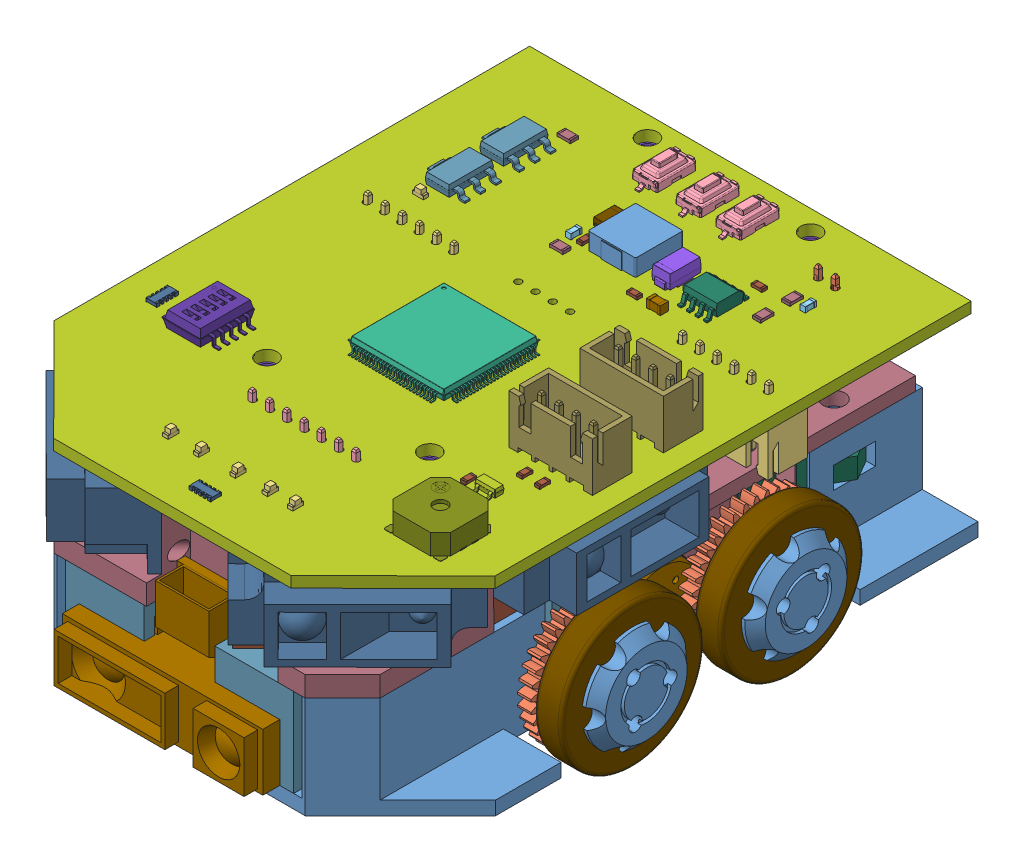
SolidWorks assembly ver 3.2, configuration Default. Lengths in mm.
Overall size (70 47.44 91.25).
236 component instances, 52 part files, 52 mates.
Components (placement in the parent):
- de 3.2-1: de 3.2 [Default] at (33.377 40.5067 64.4945) size (65 15 85)
- pin7.4v 2000mAh 30C-1: pin7.4v 2000mAh 30C [Default] at (33.377 51.5067 19.4945) x (0 -1 0) z (-1 0 0) size (18 75 15)
- schematic (2).step-1: schematic (2).step [Default] at (212.8775 69.5067 153.3034) x (-1 0 -0.000071) z (0 1 0) size (64.97 85.02 16.13)
  - LED_0603_1608Metric.step-1: LED_0603_1608Metric.step [Default] at (188.7822 -57.8002 1.65) x (0 -1 0) z (0 0 1) size (1.6 0.8 1.1)
    - LED_0603_1608Metric-0.step-1: LED_0603_1608Metric-0.step [Default] at origin size (1.6 0.8 1.1)
  - SW_Tactile_SPST_NO_Straight_CK_PTS636Sx25SMTRLFS.step-1: SW_Tactile_SPST_NO_Straight_CK_PTS636Sx25SMTRLFS.step [Default] at (173.4 -127.275 1.65) x (0 1 0) z (0 0 1) size (8 3.7 2.55)
    - PTS636Sx25SMTRLFS.step-1: PTS636Sx25SMTRLFS.step [Default] at origin size (8 3.7 2.55)
  - C_0603_1608Metric.step-1: C_0603_1608Metric.step [Default] at (184.5722 -112.8754 1.65) x (0 1 0) z (0 0 1) size (1.6 0.8 0.8)
    - C_0603_1608Metric-1.step-1: C_0603_1608Metric-1.step [Default] at origin size (1.6 0.8 0.8)
  - LQFP-100_14x14mm_P0.5mm.step-1: LQFP-100_14x14mm_P0.5mm.step [Default] at (179.8 -89 1.65) x (-1 0 0) z (0 0 1) size (16 16 1.5)
    - LQFP_100_14x14mm_P05mm.step-1: LQFP_100_14x14mm_P05mm.step [Default] at origin size (16 16 1.5)
  - SOT-23.step-1: SOT-23.step [Default] at (158.1922 -74.0902 1.65) x (0 -1 0) z (0 0 1) size (2.5 3 1.2)
    - SOT_23.step-1: SOT_23.step [Default] at origin size (2.5 3 1.2)
  - C_0603_1608Metric.step-2: C_0603_1608Metric.step [Default] at (158 -120.8 1.65) x (0 -1 0) z (0 0 1) size (1.6 0.8 0.8)
    - C_0603_1608Metric-1.step-1: C_0603_1608Metric-1.step [Default] at origin size (1.6 0.8 0.8)
  - D_SMA.step-1: D_SMA.step [Default] at (171.575 -115 1.65) x (0 -1 0) z (0 0 1) size (5 2.7 2.22)
    - D_SMA-2.step-1: D_SMA-2.step [Default] at origin size (5 2.7 2.22)
  - C_0805_2012Metric.step-1: C_0805_2012Metric.step [Default] at (168.9622 -109.6002 1.65) size (2 1.25 1.25)
    - C_0805_2012Metric-3.step-1: C_0805_2012Metric-3.step [Default] at origin size (2 1.25 1.25)
  - LED_0603_1608Metric.step-2: LED_0603_1608Metric.step [Default] at (178.88 -57.7875 1.65) x (0 -1 0) z (0 0 1) size (1.6 0.8 1.1)
    - LED_0603_1608Metric-0.step-1: LED_0603_1608Metric-0.step [Default] at origin size (1.6 0.8 1.1)
  - R_Array_Convex_5x0603.step-1: R_Array_Convex_5x0603.step [Default] at (206.8422 -74.5602 1.65) x (-1 0 0) z (0 0 1) size (1.6 3.2 0.5)
    - R_Array_Convex_5x0603-4.step-1: R_Array_Convex_5x0603-4.step [Default] at origin size (1.6 3.2 0.5)
  - R_0603_1608Metric.step-1: R_0603_1608Metric.step [Default] at (161.05 -73.875 1.65) x (0 -1 0) z (0 0 1) size (1.6 0.8 0.45)
    - R_0603_1608Metric-5.step-1: R_0603_1608Metric-5.step [Default] at origin size (1.6 0.8 0.45)
  - R_0603_1608Metric.step-2: R_0603_1608Metric.step [Default] at (155.05 -78.75 1.65) x (0 -1 0) z (0 0 1) size (1.6 0.8 0.45)
    - R_0603_1608Metric-5.step-1: R_0603_1608Metric-5.step [Default] at origin size (1.6 0.8 0.45)
  - R_0603_1608Metric.step-3: R_0603_1608Metric.step [Default] at (157.65 -78.75 1.65) x (0 -1 0) z (0 0 1) size (1.6 0.8 0.45)
    - R_0603_1608Metric-5.step-1: R_0603_1608Metric-5.step [Default] at origin size (1.6 0.8 0.45)
  - JST - XH - Thru (V) - 4Pin - 2.54mm.step-1: JST - XH - Thru (V) - 4Pin - 2.54mm.step [Default] at (156.4 -95.1037 1.65) size (12.29 5.84 10.21)
    - JST - XH - Thru - 4Pin - 2.54mm.step-1: JST - XH - Thru - 4Pin - 2.54mm.step [Default] at origin size (12.29 5.84 10.21)
  - C_0603_1608Metric.step-3: C_0603_1608Metric.step [Default] at (169.0522 -114.6252 1.65) x (0 1 0) z (0 0 1) size (1.6 0.8 0.8)
    - C_0603_1608Metric-1.step-1: C_0603_1608Metric-1.step [Default] at origin size (1.6 0.8 0.8)
  - LED_0603_1608Metric.step-3: LED_0603_1608Metric.step [Default] at (184.2422 -57.7602 1.65) x (0 -1 0) z (0 0 1) size (1.6 0.8 1.1)
    - LED_0603_1608Metric-0.step-1: LED_0603_1608Metric-0.step [Default] at origin size (1.6 0.8 1.1)
  - R_0805_2012Metric.step-1: R_0805_2012Metric.step [Default] at (160.2 -116.4 1.65) x (0 1 0) z (0 0 1) size (2 1.2 0.45)
    - R_0805_2012Metric-6.step-1: R_0805_2012Metric-6.step [Default] at origin size (2 1.2 0.45)
  - JST - XH - Thru (V) - 4Pin - 2.54mm.step-2: JST - XH - Thru (V) - 4Pin - 2.54mm.step [Default] at (156.19 -83.5908 1.65) x (-1 0 0) z (0 0 1) size (12.29 5.84 10.21)
    - JST - XH - Thru - 4Pin - 2.54mm.step-1: JST - XH - Thru - 4Pin - 2.54mm.step [Default] at origin size (12.29 5.84 10.21)
  - R_0805_2012Metric.step-2: R_0805_2012Metric.step [Default] at (183.8822 -110.1902 1.65) x (-1 0 0) z (0 0 1) size (2 1.2 0.45)
    - R_0805_2012Metric-6.step-1: R_0805_2012Metric-6.step [Default] at origin size (2 1.2 0.45)
  - SOT-223.step-1: SOT-223.step [Default] at (200.0875 -119.57 1.65) size (7 6.5 1.7)
    - SOT_223.step-1: SOT_223.step [Default] at origin size (7 6.5 1.7)
  - SOT-223.step-2: SOT-223.step [Default] at (200.1422 -111.6002 1.65) size (7 6.5 1.7)
    - SOT_223.step-1: SOT_223.step [Default] at origin size (7 6.5 1.7)
  - R_0603_1608Metric.step-4: R_0603_1608Metric.step [Default] at (172.4222 -109.6502 1.65) size (1.6 0.8 0.45)
    - R_0603_1608Metric-5.step-1: R_0603_1608Metric-5.step [Default] at origin size (1.6 0.8 0.45)
  - LED_0603_1608Metric.step-4: LED_0603_1608Metric.step [Default] at (174.1622 -57.8202 1.65) x (0 -1 0) z (0 0 1) size (1.6 0.8 1.1)
    - LED_0603_1608Metric-0.step-1: LED_0603_1608Metric-0.step [Default] at origin size (1.6 0.8 1.1)
  - R_0805_2012Metric.step-3: R_0805_2012Metric.step [Default] at (160.2 -120.6875 1.65) x (0 1 0) z (0 0 1) size (2 1.2 0.45)
    - R_0805_2012Metric-6.step-1: R_0805_2012Metric-6.step [Default] at origin size (2 1.2 0.45)
  - R_Array_Convex_5x0603.step-2: R_Array_Convex_5x0603.step [Default] at (178.8922 -52.9602 1.65) x (0 1 0) z (0 0 1) size (1.6 3.2 0.5)
    - R_Array_Convex_5x0603-4.step-1: R_Array_Convex_5x0603-4.step [Default] at origin size (1.6 3.2 0.5)
  - SW_Tactile_SPST_NO_Straight_CK_PTS636Sx25SMTRLFS.step-2: SW_Tactile_SPST_NO_Straight_CK_PTS636Sx25SMTRLFS.step [Default] at (179.2 -127.2 1.65) x (0 1 0) z (0 0 1) size (8 3.7 2.55)
    - PTS636Sx25SMTRLFS.step-1: PTS636Sx25SMTRLFS.step [Default] at origin size (8 3.7 2.55)
  - SO-8_narrow_simple.step-1: SO-8_narrow_simple.step [Default] at (165.7508 -114.6 1.65) x (-1 0 0) z (0 0 1) size (4.8 6.2 2)
    - ASSEMBLY.step-1: ASSEMBLY.step [Default] at origin size (4.8 6.2 2)
  - SW_Tactile_SPST_NO_Straight_CK_PTS636Sx25SMTRLFS.step-3: SW_Tactile_SPST_NO_Straight_CK_PTS636Sx25SMTRLFS.step [Default] at (185.6 -127.2 1.65) x (0 1 0) z (0 0 1) size (8 3.7 2.55)
    - PTS636Sx25SMTRLFS.step-1: PTS636Sx25SMTRLFS.step [Default] at origin size (8 3.7 2.55)
  - LED_0603_1608Metric.step-5: LED_0603_1608Metric.step [Default] at (200.9422 -106.7002 1.65) x (-1 0 0) z (0 0 1) size (1.6 0.8 1.1)
    - LED_0603_1608Metric-0.step-1: LED_0603_1608Metric-0.step [Default] at origin size (1.6 0.8 1.1)
  - LED_0603_1608Metric.step-6: LED_0603_1608Metric.step [Default] at (170.4722 -57.8302 1.65) x (0 -1 0) z (0 0 1) size (1.6 0.8 1.1)
    - LED_0603_1608Metric-0.step-1: LED_0603_1608Metric-0.step [Default] at origin size (1.6 0.8 1.1)
  - GSC8530YA-16R2700.step-1: GSC8530YA-16R2700.step [Default] at (157.0222 -65.7202 1.65) x (-1 0 0) z (0 1 0) size (8.55 3.15 8.5)
    - GSC8530YA-16R2700-7.step-1: GSC8530YA-16R2700-7.step [Default] at origin size (8.55 3.15 8.5)
  - SW_DIP_SPSTx05_Slide_KingTek_DSHP05TS_W7.62mm_P1.27mm.step-1: SW_DIP_SPSTx05_Slide_KingTek_DSHP05TS_W7.62mm_P1.27mm.step [Default] at (200.1022 -74.7302 1.65) x (-1 0 0) z (0 0 1) size (8.35 7.95 2.38)
    - SW_DIP_SPSTx05_Slide_KingTek_DSHP05TS_W762mm_P127mm.step-1: SW_DIP_SPSTx05_Slide_KingTek_DSHP05TS_W762mm_P127mm.step [Default] at origin size (8.35 7.95 2.38)
  - R_0603_1608Metric.step-5: R_0603_1608Metric.step [Default] at (182.9722 -112.8652 1.65) x (0 1 0) z (0 0 1) size (1.6 0.8 0.45)
    - R_0603_1608Metric-5.step-1: R_0603_1608Metric-5.step [Default] at origin size (1.6 0.8 0.45)
  - R_0805_2012Metric.step-4: R_0805_2012Metric.step [Default] at (197.4675 -124.865 1.65) size (2 1.2 0.45)
    - R_0805_2012Metric-6.step-1: R_0805_2012Metric-6.step [Default] at origin size (2 1.2 0.45)
  - CP_EIA-3216-10_Kemet-I.step-1: CP_EIA-3216-10_Kemet-I.step [Default] at (183.3922 -117.0302 1.65) x (0 1 0) z (0 0 1) size (3.4 1.8 1.2)
    - CP_EIA_3216_10_Kemet_I.step-1: CP_EIA_3216_10_Kemet_I.step [Default] at origin size (3.4 1.8 1.2)
  - Inductor_7x7x2.5.step-1: Inductor_7x7x2.5.step [Default] at (178.1322 -115.5302 1.65) x (1 0 0) z (0 -1 0) size (7 2.6 7.2)
    - Inductor_7x7x2.5-8.step-1: Inductor_7x7x2.5-8.step [Default] at origin size (7 2.6 7.2)
  - R_0603_1608Metric.step-6: R_0603_1608Metric.step [Default] at (164.2 -119.8 1.65) x (-1 0 0) z (0 0 1) size (1.6 0.8 0.45)
    - R_0603_1608Metric-5.step-1: R_0603_1608Metric-5.step [Default] at origin size (1.6 0.8 0.45)
  - C_0603_1608Metric.step-4: C_0603_1608Metric.step [Default] at (195.3522 -91.7102 -0.05) x (1 0 0) z (0 0 -1) size (1.6 0.8 0.8)
    - C_0603_1608Metric-1.step-1: C_0603_1608Metric-1.step [Default] at origin size (1.6 0.8 0.8)
  - C_0603_1608Metric.step-5: C_0603_1608Metric.step [Default] at (180.3022 -85.9102 -0.05) x (-1 0 0) z (0 0 -1) size (1.6 0.8 0.8)
    - C_0603_1608Metric-1.step-1: C_0603_1608Metric-1.step [Default] at origin size (1.6 0.8 0.8)
  - C_0603_1608Metric.step-6: C_0603_1608Metric.step [Default] at (183.6572 -94.2302 -0.05) x (-1 0 0) z (0 0 -1) size (1.6 0.8 0.8)
    - C_0603_1608Metric-1.step-1: C_0603_1608Metric-1.step [Default] at origin size (1.6 0.8 0.8)
  - B2B-XH-A_LF__SN_.step-1: B2B-XH-A_LF__SN_.step [Default] at (159.9422 -124.9552 -0.05) x (-1 0 0) z (0 -1 0) size (7.4 10.4 5.75)
    - B2B-XH-A(LF)(SN).step-1: B2B-XH-A(LF)(SN).step [Default] at origin size (7.4 10.4 5.75)
  - R_0603_1608Metric.step-7: R_0603_1608Metric.step [Default] at (179.7 -125.6 -0.05) x (-1 0 0) z (0 0 -1) size (1.6 0.8 0.45)
    - R_0603_1608Metric-5.step-1: R_0603_1608Metric-5.step [Default] at origin size (1.6 0.8 0.45)
  - JST - XH - Thru (V) - 6Pin - 2.54mm.step-1: JST - XH - Thru (V) - 6Pin - 2.54mm.step [Default] at (197.6322 -101.9902 -0.05) x (1 0 0) z (0 0 -1) size (17.37 5.84 10.21)
    - JST - XH - Thru - 6Pin - 2.54mm.step-1: JST - XH - Thru - 6Pin - 2.54mm.step [Default] at origin size (17.37 5.84 10.21)
  - CP_EIA-3216-10_Kemet-I.step-2: CP_EIA-3216-10_Kemet-I.step [Default] at (201.5522 -117.3902 -0.05) x (1 0 0) z (0 0 -1) size (3.4 1.8 1.2)
    - CP_EIA_3216_10_Kemet_I.step-1: CP_EIA_3216_10_Kemet_I.step [Default] at origin size (3.4 1.8 1.2)
  - CP_EIA-3216-10_Kemet-I.step-3: CP_EIA-3216-10_Kemet-I.step [Default] at (177.2197 -105.6402 -0.05) x (-1 0 0) z (0 0 -1) size (3.4 1.8 1.2)
    - CP_EIA_3216_10_Kemet_I.step-1: CP_EIA_3216_10_Kemet_I.step [Default] at origin size (3.4 1.8 1.2)
  - R_0603_1608Metric.step-8: R_0603_1608Metric.step [Default] at (174.2 -125.475 -0.05) x (-1 0 0) z (0 0 -1) size (1.6 0.8 0.45)
    - R_0603_1608Metric-5.step-1: R_0603_1608Metric-5.step [Default] at origin size (1.6 0.8 0.45)
  - C_0603_1608Metric.step-7: C_0603_1608Metric.step [Default] at (183.6972 -92.4602 -0.05) x (-1 0 0) z (0 0 -1) size (1.6 0.8 0.8)
    - C_0603_1608Metric-1.step-1: C_0603_1608Metric-1.step [Default] at origin size (1.6 0.8 0.8)
  - CP_EIA-3216-10_Kemet-I.step-4: CP_EIA-3216-10_Kemet-I.step [Default] at (171.2722 -117.1002 -0.05) x (0 -1 0) z (0 0 -1) size (3.4 1.8 1.2)
    - CP_EIA_3216_10_Kemet_I.step-1: CP_EIA_3216_10_Kemet_I.step [Default] at origin size (3.4 1.8 1.2)
  - C_0603_1608Metric.step-8: C_0603_1608Metric.step [Default] at (184.8 -125.6 -0.05) x (1 0 0) z (0 0 -1) size (1.6 0.8 0.8)
    - C_0603_1608Metric-1.step-1: C_0603_1608Metric-1.step [Default] at origin size (1.6 0.8 0.8)
  - JST - XH - Thru (V) - 6Pin - 2.54mm.step-2: JST - XH - Thru (V) - 6Pin - 2.54mm.step [Default] at (156.6722 -107.3602 -0.05) x (1 0 0) z (0 0 -1) size (17.37 5.84 10.21)
    - JST - XH - Thru - 6Pin - 2.54mm.step-1: JST - XH - Thru - 6Pin - 2.54mm.step [Default] at origin size (17.37 5.84 10.21)
  - C_0603_1608Metric.step-9: C_0603_1608Metric.step [Default] at (177.5197 -107.4902 -0.05) x (-1 0 0) z (0 0 -1) size (1.6 0.8 0.8)
    - C_0603_1608Metric-1.step-1: C_0603_1608Metric-1.step [Default] at origin size (1.6 0.8 0.8)
  - JST - XH - Thru (V) - 7Pin - 2.54mm.step-1: JST - XH - Thru (V) - 7Pin - 2.54mm.step [Default] at (179.7522 -68.3802 -0.05) x (1 0 0) z (0 0 -1) size (19.91 5.84 10.21)
    - JST - XH - Thru - 7Pin - 2.54mm.step-1: JST - XH - Thru - 7Pin - 2.54mm.step [Default] at origin size (19.91 5.84 10.21)
  - C_0603_1608Metric.step-10: C_0603_1608Metric.step [Default] at (180.31 -87.58 -0.05) x (-1 0 0) z (0 0 -1) size (1.6 0.8 0.8)
    - C_0603_1608Metric-1.step-1: C_0603_1608Metric-1.step [Default] at origin size (1.6 0.8 0.8)
  - C_0603_1608Metric.step-11: C_0603_1608Metric.step [Default] at (183.6272 -88.9602 -0.05) x (-1 0 0) z (0 0 -1) size (1.6 0.8 0.8)
    - C_0603_1608Metric-1.step-1: C_0603_1608Metric-1.step [Default] at origin size (1.6 0.8 0.8)
  - CP_EIA-3216-10_Kemet-I.step-5: CP_EIA-3216-10_Kemet-I.step [Default] at (201.5422 -113.8002 -0.05) x (1 0 0) z (0 0 -1) size (3.4 1.8 1.2)
    - CP_EIA_3216_10_Kemet_I.step-1: CP_EIA_3216_10_Kemet_I.step [Default] at origin size (3.4 1.8 1.2)
  - R_0603_1608Metric.step-9: R_0603_1608Metric.step [Default] at (160.18 -91.9945 -0.05) x (0 1 0) z (0 0 -1) size (1.6 0.8 0.45)
    - R_0603_1608Metric-5.step-1: R_0603_1608Metric-5.step [Default] at origin size (1.6 0.8 0.45)
  - C_0603_1608Metric.step-12: C_0603_1608Metric.step [Default] at (183.5822 -85.8802 -0.05) x (1 0 0) z (0 0 -1) size (1.6 0.8 0.8)
    - C_0603_1608Metric-1.step-1: C_0603_1608Metric-1.step [Default] at origin size (1.6 0.8 0.8)
  - C_0603_1608Metric.step-13: C_0603_1608Metric.step [Default] at (175.4 -92.9 -0.05) x (1 0 0) z (0 0 -1) size (1.6 0.8 0.8)
    - C_0603_1608Metric-1.step-1: C_0603_1608Metric-1.step [Default] at origin size (1.6 0.8 0.8)
  - C_0603_1608Metric.step-14: C_0603_1608Metric.step [Default] at (195.4222 -86.5502 -0.05) x (1 0 0) z (0 0 -1) size (1.6 0.8 0.8)
    - C_0603_1608Metric-1.step-1: C_0603_1608Metric-1.step [Default] at origin size (1.6 0.8 0.8)
  - C_0603_1608Metric.step-15: C_0603_1608Metric.step [Default] at (183.6122 -84.1702 -0.05) x (1 0 0) z (0 0 -1) size (1.6 0.8 0.8)
    - C_0603_1608Metric-1.step-1: C_0603_1608Metric-1.step [Default] at origin size (1.6 0.8 0.8)
  - R_0603_1608Metric.step-10: R_0603_1608Metric.step [Default] at (200.5422 -109.4502 -0.05) x (-1 0 0) z (0 0 -1) size (1.6 0.8 0.45)
    - R_0603_1608Metric-5.step-1: R_0603_1608Metric-5.step [Default] at origin size (1.6 0.8 0.45)
  - Crystal_SMD_3225-4Pin_3.2x2.5mm.step-1: Crystal_SMD_3225-4Pin_3.2x2.5mm.step [Default] at (195.4222 -89.2002 -0.05) x (1 0 0) z (0 0 -1) size (3.2 2.5 0.64)
    - Crystal_SMD_3225-4Pin_3.2x2.5mm-9.step-1: Crystal_SMD_3225-4Pin_3.2x2.5mm-9.step [Default] at origin size (3.2 2.5 0.64)
  - C_0603_1608Metric.step-16: C_0603_1608Metric.step [Default] at (183.6 -82.6 -0.05) x (-1 0 0) z (0 0 -1) size (1.6 0.8 0.8)
    - C_0603_1608Metric-1.step-1: C_0603_1608Metric-1.step [Default] at origin size (1.6 0.8 0.8)
  - R_0603_1608Metric.step-11: R_0603_1608Metric.step [Default] at (157.68 -91.9445 -0.05) x (0 -1 0) z (0 0 -1) size (1.6 0.8 0.45)
    - R_0603_1608Metric-5.step-1: R_0603_1608Metric-5.step [Default] at origin size (1.6 0.8 0.45)
  - C_0603_1608Metric.step-17: C_0603_1608Metric.step [Default] at (179.7 -128.5 -0.05) x (-1 0 0) z (0 0 -1) size (1.6 0.8 0.8)
    - C_0603_1608Metric-1.step-1: C_0603_1608Metric-1.step [Default] at origin size (1.6 0.8 0.8)
  - R_0603_1608Metric.step-12: R_0603_1608Metric.step [Default] at (183.7 -97.3 -0.05) x (-1 0 0) z (0 0 -1) size (1.6 0.8 0.45)
    - R_0603_1608Metric-5.step-1: R_0603_1608Metric-5.step [Default] at origin size (1.6 0.8 0.45)
  - C_0603_1608Metric.step-18: C_0603_1608Metric.step [Default] at (174.2 -128.275 -0.05) x (-1 0 0) z (0 0 -1) size (1.6 0.8 0.8)
    - C_0603_1608Metric-1.step-1: C_0603_1608Metric-1.step [Default] at origin size (1.6 0.8 0.8)
  - C_0603_1608Metric.step-19: C_0603_1608Metric.step [Default] at (183.6 -90.7 -0.05) x (-1 0 0) z (0 0 -1) size (1.6 0.8 0.8)
    - C_0603_1608Metric-1.step-1: C_0603_1608Metric-1.step [Default] at origin size (1.6 0.8 0.8)
  - CP_EIA-3216-10_Kemet-I.step-6: CP_EIA-3216-10_Kemet-I.step [Default] at (201.5422 -111.5502 -0.05) x (1 0 0) z (0 0 -1) size (3.4 1.8 1.2)
    - CP_EIA_3216_10_Kemet_I.step-1: CP_EIA_3216_10_Kemet_I.step [Default] at origin size (3.4 1.8 1.2)
  - C_0603_1608Metric.step-20: C_0603_1608Metric.step [Default] at (152.48 -91.8945 -0.05) x (0 1 0) z (0 0 -1) size (1.6 0.8 0.8)
    - C_0603_1608Metric-1.step-1: C_0603_1608Metric-1.step [Default] at origin size (1.6 0.8 0.8)
  - C_0603_1608Metric.step-21: C_0603_1608Metric.step [Default] at (176.7 -85.4 -0.05) x (1 0 0) z (0 0 -1) size (1.6 0.8 0.8)
    - C_0603_1608Metric-1.step-1: C_0603_1608Metric-1.step [Default] at origin size (1.6 0.8 0.8)
  - C_0603_1608Metric.step-22: C_0603_1608Metric.step [Default] at (176.7 -83.7 -0.05) x (1 0 0) z (0 0 -1) size (1.6 0.8 0.8)
    - C_0603_1608Metric-1.step-1: C_0603_1608Metric-1.step [Default] at origin size (1.6 0.8 0.8)
  - C_0603_1608Metric.step-23: C_0603_1608Metric.step [Default] at (175.4 -94.5 -0.05) x (1 0 0) z (0 0 -1) size (1.6 0.8 0.8)
    - C_0603_1608Metric-1.step-1: C_0603_1608Metric-1.step [Default] at origin size (1.6 0.8 0.8)
  - CP_EIA-3216-10_Kemet-I.step-7: CP_EIA-3216-10_Kemet-I.step [Default] at (201.5375 -122.02 -0.05) x (1 0 0) z (0 0 -1) size (3.4 1.8 1.2)
    - CP_EIA_3216_10_Kemet_I.step-1: CP_EIA_3216_10_Kemet_I.step [Default] at origin size (3.4 1.8 1.2)
  - C_0603_1608Metric.step-24: C_0603_1608Metric.step [Default] at (173.1722 -116.6002 -0.05) x (0 -1 0) z (0 0 -1) size (1.6 0.8 0.8)
    - C_0603_1608Metric-1.step-1: C_0603_1608Metric-1.step [Default] at origin size (1.6 0.8 0.8)
  - SSOP-24_5.3x8.2mm_P0.65mm.step-1: SSOP-24_5.3x8.2mm_P0.65mm.step [Default] at (178.875 -116.225 -0.05) x (0 1 0) z (0 0 -1) size (7.8 8.2 2.1)
    - SSOP_24_53x82mm_P065mm.step-1: SSOP_24_53x82mm_P065mm.step [Default] at origin size (7.8 8.2 2.1)
  - schematic_PCB.step-1: schematic_PCB.step [Default] at origin size (64.97 85.02 1.6)
- truc dong cai cai 30mm-1: truc dong cai cai 30mm [По умолчанию] at (45.2628 49.5067 78.5514) size (5 20 5.77)
- truc dong cai cai 30mm-2: truc dong cai cai 30mm [По умолчанию] at (45.2768 49.5067 22.5211) size (5 20 5.77)
- truc dong cai cai 30mm-3: truc dong cai cai 30mm [По умолчанию] at (21.2568 49.5067 22.5194) size (5 20 5.77)
- truc dong cai cai 30mm-4: truc dong cai cai 30mm [По умолчанию] at (21.2628 49.5067 78.5094) size (5 20 5.77)
- GP2Y0A41SK0F-1: GP2Y0A41SK0F [Default] at (33.377 46.7067 94.4945) x (-1 0 0) z (0 0 1) size (29.5 18.9 13.5)
- SHARP GP2Y0A51SK0F.step-2: SHARP GP2Y0A51SK0F.step [Default] at (30.2161 81.6771 68.4074) x (0.000071 0 -1) z (0 -1 0) size (27 14.5 13.5)
  - шарп крышка.step-1: шарп крышка.step [Default] at (-12.8819 -17.3225 12.1705) x (1 0 0) z (0 -1 0) size (27 11 12)
  - шарп плата.step-1: шарп плата.step [Default] at (13.6181 -19.3225 25.6705) x (-1 0 0) z (0 -1 0) size (26 13 5.5)
  - 92000A010_Passivated 18-8 Stainless Steel Pan Head Phillips Screws.step-1: 92000A010_Passivated 18-8 Stainless Steel Pan Head Phillips Screws.step [Default] at (11.4181 -22.3225 19.1705) x (1 0 0) z (0 1 0) size (4 4 4.61)
  - 92000A010_Passivated 18-8 Stainless Steel Pan Head Phillips Screws.step-2: 92000A010_Passivated 18-8 Stainless Steel Pan Head Phillips Screws.step [Default] at (-10.1819 -22.3225 14.8705) x (1 0 0) z (0 1 0) size (4 4 4.61)
- SHARP GP2Y0A51SK0F.step-3: SHARP GP2Y0A51SK0F.step [Default] at (36.5366 81.6771 67.1717) x (-0.000071 0 1) z (0 -1 0) size (27 14.5 13.5)
  - шарп крышка.step-1: шарп крышка.step [Default] at (-12.8819 -17.3225 12.1705) x (1 0 0) z (0 -1 0) size (27 11 12)
  - шарп плата.step-1: шарп плата.step [Default] at (13.6181 -19.3225 25.6705) x (-1 0 0) z (0 -1 0) size (26 13 5.5)
  - 92000A010_Passivated 18-8 Stainless Steel Pan Head Phillips Screws.step-1: 92000A010_Passivated 18-8 Stainless Steel Pan Head Phillips Screws.step [Default] at (11.4181 -22.3225 19.1705) x (1 0 0) z (0 1 0) size (4 4 4.61)
  - 92000A010_Passivated 18-8 Stainless Steel Pan Head Phillips Screws.step-2: 92000A010_Passivated 18-8 Stainless Steel Pan Head Phillips Screws.step [Default] at (-10.1819 -22.3225 14.8705) x (1 0 0) z (0 1 0) size (4 4 4.61)
- SHARP GP2Y0A51SK0F.step-4: SHARP GP2Y0A51SK0F.step [Default] at (36.0247 81.6771 79.0059) x (-0.708334 0 0.705877) z (0 -1 0) size (27 14.5 13.5)
  - шарп крышка.step-1: шарп крышка.step [Default] at (-12.8819 -17.3225 12.1705) x (1 0 0) z (0 -1 0) size (27 11 12)
  - шарп плата.step-1: шарп плата.step [Default] at (13.6181 -19.3225 25.6705) x (-1 0 0) z (0 -1 0) size (26 13 5.5)
  - 92000A010_Passivated 18-8 Stainless Steel Pan Head Phillips Screws.step-1: 92000A010_Passivated 18-8 Stainless Steel Pan Head Phillips Screws.step [Default] at (11.4181 -22.3225 19.1705) x (1 0 0) z (0 1 0) size (4 4 4.61)
  - 92000A010_Passivated 18-8 Stainless Steel Pan Head Phillips Screws.step-2: 92000A010_Passivated 18-8 Stainless Steel Pan Head Phillips Screws.step [Default] at (-10.1819 -22.3225 14.8705) x (1 0 0) z (0 1 0) size (4 4 4.61)
- SHARP GP2Y0A51SK0F.step-5: SHARP GP2Y0A51SK0F.step [Default] at (31.6049 81.6771 79.8784) x (-0.708334 0 -0.705877) z (0 -1 0) size (27 14.5 13.5)
  - шарп крышка.step-1: шарп крышка.step [Default] at (-12.8819 -17.3225 12.1705) x (1 0 0) z (0 -1 0) size (27 11 12)
  - шарп плата.step-1: шарп плата.step [Default] at (13.6181 -19.3225 25.6705) x (-1 0 0) z (0 -1 0) size (26 13 5.5)
  - 92000A010_Passivated 18-8 Stainless Steel Pan Head Phillips Screws.step-1: 92000A010_Passivated 18-8 Stainless Steel Pan Head Phillips Screws.step [Default] at (11.4181 -22.3225 19.1705) x (1 0 0) z (0 1 0) size (4 4 4.61)
  - 92000A010_Passivated 18-8 Stainless Steel Pan Head Phillips Screws.step-2: 92000A010_Passivated 18-8 Stainless Steel Pan Head Phillips Screws.step [Default] at (-10.1819 -22.3225 14.8705) x (1 0 0) z (0 1 0) size (4 4 4.61)
- Cum 1-1: Cum 1 [Default] at (38.2699 36.5628 69.5041) x (0 0 -1) z (1 0 0) size (51.81 29.03 26.81)
  - Tach 1-1: Tach 1 [Default] at (11.4596 10.9438 19.4071) x (-1 0 0) z (0 0 -1) size (24.5 15 9)
  - Tach 2-1: Tach 2 [Default] at (11.4596 10.9438 19.4071) x (-1 0 0) z (0 0 -1) size (8.5 15 9)
  - Tach 3-1: Tach 3 [Default] at (11.4596 10.9438 19.4071) x (-1 0 0) z (0 0 -1) size (16.1 15 9)
  - Vong bi 2x5x2.5-1: Vong bi 2x5x2.5 [Default] at (-0.2904 10.9438 17.5163) x (-0.56855 -0.822648 0) z (0 0 1) size (5 5 3)
  - Vong bi 2x5x2.5-2: Vong bi 2x5x2.5 [Default] at (23.2096 10.9438 17.5163) size (5 5 3)
  - Vong bi 2x5x2.5-3: Vong bi 2x5x2.5 [Default] at (-0.2904 10.9438 20.5163) x (0.682135 -0.731226 0) z (0 0 1) size (5 5 3)
  - Vong bi 2x5x2.5-4: Vong bi 2x5x2.5 [Default] at (23.2096 10.9438 20.5163) x (0.791447 0.611238 0) z (0 0 1) size (5 5 3)
  - Phanh kep truc 8mm-1: Phanh kep truc 8mm [Default] at (23.2096 10.9438 19.9071) x (0 1 0) z (0 0 1) size (10 11.12 0.4)
  - Phanh kep truc 8mm-2: Phanh kep truc 8mm [Default] at (-0.2904 10.9438 19.9071) x (0 -1 0) z (0 0 1) size (10 11.12 0.4)
  - Phanh kep truc 8mm-3: Phanh kep truc 8mm [Default] at (-0.2904 10.9438 12.9071) x (0 -1 0) z (0 0 1) size (10 11.12 0.4)
  - Phanh kep truc 8mm-4: Phanh kep truc 8mm [Default] at (23.2096 10.9438 12.9071) x (0 1 0) z (0 0 1) size (10 11.12 0.4)
  - Banh xe-1: Banh xe [Default] at (11.0671 17.3903 4.8282) x (0 0 1) z (0.970821 0.239806 0) size (20 27.44 27.43)
    - Lop banh xe-2: Lop banh xe [Default] at (18.2789 9.1703 10.2423) size (4 21 21)
    - Mam Banh xe-2: Mam Banh xe [Default] at (18.2789 9.1703 10.2423) size (7 15.03 15)
    - Spur gear 0.5M 38T V2.4.2-2: Spur gear 0.5M 38T V2.4.2 [Default] at (18.2789 9.1703 10.2423) x (-1 0 0) z (0 -0.855409 0.517953) size (2 19.95 20)
    - Truc 2x20-2: Truc 2x20 [Default] at (14.2789 9.1703 10.2423) x (0 0.207598 -0.978214) z (1 0 0) size (2 2 18)
  - Banh xe-2: Banh xe [Default] at (13.2866 8.7842 4.8282) x (0 0 1) z (-0.840559 -0.54172 0) size (20 27.44 27.43)
    - Lop banh xe-2: Lop banh xe [Default] at (18.2789 9.1703 10.2423) size (4 21 21)
    - Mam Banh xe-2: Mam Banh xe [Default] at (18.2789 9.1703 10.2423) size (7 15.03 15)
    - Spur gear 0.5M 38T V2.4.2-2: Spur gear 0.5M 38T V2.4.2 [Default] at (18.2789 9.1703 10.2423) x (-1 0 0) z (0 -0.855409 0.517953) size (2 19.95 20)
    - Truc 2x20-2: Truc 2x20 [Default] at (14.2789 9.1703 10.2423) x (0 0.207598 -0.978214) z (1 0 0) size (2 2 18)
  - Ga encoder 1 V2.4.2-1: Ga encoder 1 V2.4.2 [Default] at (23.3096 14.6438 6.9071) x (-1 0 0) z (0 -1 0) size (23 14.5 16.6)
  - Ga nam chamV3-1: Ga nam chamV3 [Default] at (-0.2904 10.9438 12.6071) x (0 0 -1) z (1 0 0) size (2.5 4.5 4.5)
  - Ga nam chamV3.1-1: Ga nam chamV3.1 [Default] at (23.2096 10.9438 13.1071) x (0 0 -1) z (0.039989 0.9992 0) size (5 7.5 7.5)
  - Nam cham-1: Nam cham [Default] at (23.2096 10.9438 9.1071) x (0.893121 0.449816 0) z (0 0 1) size (4 4 2)
  - MT6701 Ver2-1: MT6701 Ver2 [Default] at (23.1096 11.6134 3.2971) x (-1 0 0) z (0 0 1) size (23 17.5 3.61)
  - N20 DC MOTOR Truc dai-1: N20 DC MOTOR Truc dai [Default] at (11.4595 10.8644 5.3071) x (0 1 0) z (1 0 0) size (12.48 22.6 10.65)
- cum 2-1: cum 2 [Default] at (28.7923 33.3565 48.5883) x (0 0 1) z (-1 0 0) size (51.34 28.08 26.8)
  - Tach 1-1: Tach 1 [Default] at (9.4562 14.1502 13.7153) size (24.5 15 9)
  - Tach 2-1: Tach 2 [Default] at (9.4562 14.1502 13.7153) size (8.5 15 9)
  - Tach 4-1: Tach 4 [Default] at (9.4562 14.1502 13.7153) size (16.1 15 9)
  - Ga encoder 2 V2.4.2-1: Ga encoder 2 V2.4.2 [Default] at (-2.3938 17.9502 5.2153) x (1 0 0) z (0 -1 0) size (23 14.5 16.6)
  - N20 DC MOTOR Truc dai-1: N20 DC MOTOR Truc dai [Default] at (9.4561 14.0708 5.6153) x (0 1 0) z (1 0 0) size (12.48 22.6 10.65)
  - MT6701 Ver3-1: MT6701 Ver3 [Default] at (-2.1938 14.9198 3.6153) x (-1 0 0) z (0 0 1) size (23 17.5 3.61)
  - Banh xe-1: Banh xe [Default] at (30.1673 3.7244 5.1364) x (0 0 1) z (-0.991487 0.130203 0) size (20 27.44 27.43)
    - Lop banh xe-2: Lop banh xe [Default] at (18.2789 9.1703 10.2423) size (4 21 21)
    - Mam Banh xe-2: Mam Banh xe [Default] at (18.2789 9.1703 10.2423) size (7 15.03 15)
    - Spur gear 0.5M 38T V2.4.2-2: Spur gear 0.5M 38T V2.4.2 [Default] at (18.2789 9.1703 10.2423) x (-1 0 0) z (0 -0.855409 0.517953) size (2 19.95 20)
    - Truc 2x20-2: Truc 2x20 [Default] at (14.2789 9.1703 10.2423) x (0 0.207598 -0.978214) z (1 0 0) size (2 2 18)
  - Banh xe-2: Banh xe [Default] at (8.5875 5.748 5.1364) x (0 0 1) z (-0.997359 -0.072628 0) size (20 27.44 27.43)
    - Lop banh xe-2: Lop banh xe [Default] at (18.2789 9.1703 10.2423) size (4 21 21)
    - Mam Banh xe-2: Mam Banh xe [Default] at (18.2789 9.1703 10.2423) size (7 15.03 15)
    - Spur gear 0.5M 38T V2.4.2-2: Spur gear 0.5M 38T V2.4.2 [Default] at (18.2789 9.1703 10.2423) x (-1 0 0) z (0 -0.855409 0.517953) size (2 19.95 20)
    - Truc 2x20-2: Truc 2x20 [Default] at (14.2789 9.1703 10.2423) x (0 0.207598 -0.978214) z (1 0 0) size (2 2 18)
  - Phanh kep truc 8mm-1: Phanh kep truc 8mm [Default] at (-2.0739 14.1502 13.3137) x (0 -1 0) z (0 0 1) size (10 11.12 0.4)
  - Phanh kep truc 8mm-2: Phanh kep truc 8mm [Default] at (21.1362 14.1502 13.3137) x (0 -1 0) z (0 0 -1) size (10 11.12 0.4)
  - Ga nam chamV3-1: Ga nam chamV3 [Default] at (21.2062 14.1502 12.9153) x (0 0 -1) z (1 0 0) size (2.5 4.5 4.5)
  - Ga nam chamV3.1-1: Ga nam chamV3.1 [Default] at (-2.2938 14.1502 13.2253) x (0 0 -1) z (-0.643351 0.765571 0) size (5 7.5 7.5)
  - Nam cham-1: Nam cham [Default] at (-2.2938 14.1502 9.2253) size (4 4 2)
- ga 2-1: ga 2 [Default] at (33.377 55.5067 19.4945) size (48.6 14 84) (hidden)
- ga 1-2: ga 1 [Default] at (33.377 42.5067 94.6445) x (0 0 1) z (-1 0 0) size (8.85 13 39.6)
- daioc 3-1: daioc 3 [Default] at (12.077 49.0067 28.4945) x (0.508626 0 0.860988) z (-0.860988 0 0.508626) size (6.93 3 6.03)
- daioc 3-2: daioc 3 [Default] at (54.677 49.0067 28.4945) x (0.99995 0 -0.009989) z (0.009989 0 0.99995) size (6.93 3 6.03)
- ga3-1: ga3 [Default] at (33.377 42.5067 18.4945) x (-1 0 0) z (0 0 -1) size (46.5 13 5.8)
Mates (geometry in assembly coordinates):
- Coincident1: coincident anti-aligned: plane of de 3.2-1 through (33.377 42.5067 64.4945) normal (0 1 0); plane of Cum 1-1/Tach 3-1 through (51.677 42.5067 58.0445) normal (0 -1 0)
- Coincident2: coincident anti-aligned: plane of de 3.2-1 through (33.377 42.5067 64.4945) normal (0 1 0); plane of cum 2-1/Tach 4-1 through (9.077 42.5067 58.0445) normal (0 -1 0)
- Distance1: distance = 13 mm aligned: plane of cum 2-1/Tach 4-1 through (9.077 38.9011 32.4945) normal (0 0 -1); plane of de 3.2-1 through (0.877 42.5067 19.4945) normal (0 0 -1)
- Distance2: distance = 0.5 mm aligned: plane of cum 2-1/Banh xe-2/Lop banh xe-2 through (0.377 57.9789 45.5319) normal (-1 0 0); plane of de 3.2-1 through (0.877 42.5067 109.4945) normal (-1 0 0)
- Distance3: distance = 13 mm aligned: plane of Cum 1-1/Tach 3-1 through (51.677 38.9011 32.4945) normal (0 0 -1); plane of de 3.2-1 through (0.877 42.5067 19.4945) normal (0 0 -1)
- Distance4: distance = 0.5 mm aligned: plane of Cum 1-1/Banh xe-1/Lop banh xe-2 through (66.377 37.313 43.7765) normal (1 0 0); plane of de 3.2-1 through (65.877 42.5067 109.4945) normal (1 0 0)
- Coincident7: coincident anti-aligned: plane of de 3.2-1 through (33.377 42.5067 64.4945) normal (0 1 0); plane of pin7.4v 2000mAh 30C-1 through (25.877 42.5067 94.4945) normal (0 -1 0)
- Width1: width anti-aligned: plane of pin7.4v 2000mAh 30C-1 through (40.877 60.5067 94.4945) normal (1 0 0); plane of pin7.4v 2000mAh 30C-1 through (25.877 60.5067 94.4945) normal (-1 0 0); plane of de 3.2-1 through (0.877 42.5067 109.4945) normal (-1 0 0); plane of de 3.2-1 through (65.877 42.5067 109.4945) normal (1 0 0)
- Coincident10: coincident aligned: plane of de 3.2-1 through (0.877 42.5067 19.4945) normal (0 0 -1); plane of pin7.4v 2000mAh 30C-1 through (33.377 51.5067 19.4945) normal (0 0 -1)
- Coincident12: coincident anti-aligned: plane of pin7.4v 2000mAh 30C-1 through (33.377 51.5067 94.4945) normal (0 0 1); plane of GP2Y0A41SK0F-1 through (43.627 46.7067 94.4945) normal (0 0 -1)
- Width2: width anti-aligned: plane of GP2Y0A41SK0F-1 through (18.627 50.9067 94.4945) normal (-1 0 0); plane of GP2Y0A41SK0F-1 through (48.127 42.5067 94.4945) normal (1 0 0); plane of de 3.2-1 through (65.877 42.5067 109.4945) normal (1 0 0); plane of de 3.2-1 through (0.877 42.5067 109.4945) normal (-1 0 0)
- Coincident31: coincident aligned: plane of SHARP GP2Y0A51SK0F.step-2/шарп крышка.step-1 through (12.8945 69.5067 54.2881) normal (0.000071 0 -1); plane of SHARP GP2Y0A51SK0F.step-3/шарп крышка.step-1 through (53.8601 58.5067 54.291) normal (0.000071 0 -1)
- Coincident32: coincident anti-aligned: plane of de 3.2-1 through (33.377 42.5067 64.4945) normal (0 1 0); plane of GP2Y0A41SK0F-1 through (18.627 42.5067 94.4945) normal (0 -1 0)
- Distance12: distance = 0.5 mm anti-aligned: plane of SHARP GP2Y0A51SK0F.step-3/шарп плата.step-1 through (55.8582 56.0067 80.7912) normal (0 -1 0); plane of de 3.2-1 through (33.377 55.5067 64.4945) normal (0 1 0)
- Distance13: distance = 27 mm anti-aligned: plane of schematic (2).step-1/schematic_PCB.step-1 through (212.8775 69.5067 153.3034) normal (0 -1 0); plane of de 3.2-1 through (33.377 42.5067 64.4945) normal (0 1 0)
- Width3: width aligned: plane of schematic (2).step-1/schematic_PCB.step-1 through (0.892 69.5067 89.4838) normal (-1 0 -0.000071); plane of de 3.2-1 through (65.857 69.5067 19.4984) normal (1 0 -0.000071); plane of schematic (2).step-1/schematic_PCB.step-1 through (65.877 42.5067 109.4945) normal (1 0 0); plane of de 3.2-1 through (0.877 42.5067 109.4945) normal (-1 0 0)
- Coincident35: coincident anti-aligned: plane of SHARP GP2Y0A51SK0F.step-2/шарп крышка.step-1 through (12.8926 69.5067 81.2881) normal (0 1 0); plane of schematic (2).step-1/schematic_PCB.step-1 through (212.8775 69.5067 153.3034) normal (0 -1 0)
- Distance14: distance = 0.5 mm anti-aligned: plane of SHARP GP2Y0A51SK0F.step-2/шарп крышка.step-1 through (12.8945 69.5067 54.2881) normal (0.000071 0 -1); plane of schematic (2).step-1/JST - XH - Thru (V) - 6Pin - 2.54mm.step-1/JST - XH - Thru - 6Pin - 2.54mm.step-1 through (6.5656 68.7455 53.7876) normal (-0.000071 0 1)
- Coincident40: coincident aligned: plane of SHARP GP2Y0A51SK0F.step-2/шарп крышка.step-1 through (0.8936 64.0067 67.7872) normal (-1 0 -0.000071); plane of schematic (2).step-1/schematic_PCB.step-1 through (0.892 69.5067 89.4838) normal (-1 0 -0.000071)
- Coincident43: coincident: point of SHARP GP2Y0A51SK0F.step-3/шарп крышка.step-1; plane of schematic (2).step-1/schematic_PCB.step-1 through (65.857 69.5067 19.4984) normal (1 0 -0.000071)
- Coincident49: coincident anti-aligned: plane of schematic (2).step-1/schematic_PCB.step-1 through (212.8775 69.5067 153.3034) normal (0 -1 0); plane of truc dong cai cai 30mm-3 through (21.2568 69.5067 22.5194) normal (0 1 0)
- Concentric1: concentric anti-aligned: cylinder of schematic (2).step-1/schematic_PCB.step-1 through (21.2568 69.5067 22.5194) axis (0 -1 0) radius 1.5003; cylinder of truc dong cai cai 30mm-3 through (21.2568 69.5067 22.5194) axis (0 1 0) radius 1.25
- Coincident50: coincident anti-aligned: plane of schematic (2).step-1/schematic_PCB.step-1 through (212.8775 69.5067 153.3034) normal (0 -1 0); plane of truc dong cai cai 30mm-2 through (45.2768 69.5067 22.5211) normal (0 1 0)
- Concentric2: concentric aligned: circle of schematic (2).step-1/schematic_PCB.step-1; cylinder of truc dong cai cai 30mm-2 through (45.2768 69.5067 22.5211) axis (0 1 0) radius 1.25
- Coincident51: coincident anti-aligned: plane of schematic (2).step-1/schematic_PCB.step-1 through (212.8775 69.5067 153.3034) normal (0 -1 0); plane of truc dong cai cai 30mm-4 through (21.2628 69.5067 78.5094) normal (0 1 0)
- Coincident52: coincident anti-aligned: plane of schematic (2).step-1/schematic_PCB.step-1 through (212.8775 69.5067 153.3034) normal (0 -1 0); plane of truc dong cai cai 30mm-1 through (45.2628 69.5067 78.5514) normal (0 1 0)
- Concentric3: concentric anti-aligned: cylinder of schematic (2).step-1/schematic_PCB.step-1 through (21.2628 69.5067 78.5094) axis (0 -1 0) radius 1.5003; cylinder of truc dong cai cai 30mm-4 through (21.2628 69.5067 78.5094) axis (0 1 0) radius 1.25
- Concentric4: concentric anti-aligned: cylinder of schematic (2).step-1/schematic_PCB.step-1 through (45.2628 69.5067 78.5514) axis (0 -1 0) radius 1.5; cylinder of truc dong cai cai 30mm-1 through (45.2628 69.5067 78.5514) axis (0 1 0) radius 1.25
- Width8: width anti-aligned: plane of ga 2-1 through (57.377 58.5067 97.9945) normal (1 0 0); plane of de 3.2-1 through (9.377 58.5067 97.9945) normal (-1 0 0); plane of ga 2-1 through (9.377 32.5067 79.8445) normal (-1 0 0); plane of de 3.2-1 through (57.377 32.5067 79.8445) normal (1 0 0)
- Coincident55: coincident aligned: plane of ga 2-1 through (33.377 69.5067 19.4945) normal (0 1 0); plane of SHARP GP2Y0A51SK0F.step-5/шарп крышка.step-1 through (28.5021 69.5067 101.2416) normal (0 1 0)
- Coincident56: coincident anti-aligned: plane of ga 2-1 through (-9.9253 69.5067 62.9476) normal (-0.705877 0 0.708334); plane of SHARP GP2Y0A51SK0F.step-5/шарп крышка.step-1 through (18.9395 64.0067 91.7123) normal (0.705877 0 -0.708334)
- Coincident58: coincident: line of ga 2-1 through (9.377 69.5067 82.183) axis (0 -1 0); plane of SHARP GP2Y0A51SK0F.step-5/шарп крышка.step-1 through (9.377 69.5067 82.183) normal (-0.708334 0 -0.705877)
- Coincident61: coincident anti-aligned: plane of SHARP GP2Y0A51SK0F.step-4/шарп крышка.step-1 through (47.8145 64.0067 91.7123) normal (-0.705877 0 -0.708334); plane of ga 2-1 through (76.6794 69.5067 62.9476) normal (0.705877 0 0.708334)
- Coincident62: coincident: line of SHARP GP2Y0A51SK0F.step-4/шарп крышка.step-1 through (57.377 58.5067 82.183) axis (0 1 0); plane of ga 2-1 through (57.377 58.5067 97.9945) normal (1 0 0)
- Coincident63: coincident aligned: plane of SHARP GP2Y0A51SK0F.step-4/шарп крышка.step-1 through (57.377 69.5067 82.183) normal (0 1 0); plane of ga 2-1 through (33.377 69.5067 19.4945) normal (0 1 0)
- Coincident64: coincident anti-aligned: plane of de 3.2-1 through (33.377 42.5067 64.4945) normal (0 1 0); plane of ga 1-2 through (53.377 42.5067 97.6445) normal (0 -1 0)
- Coincident66: coincident aligned: plane of de 3.2-1 through (0.877 42.5067 19.4945) normal (0 0 -1); plane of ga 2-1 through (57.377 58.5067 19.4945) normal (0 0 -1)
- Width11: width anti-aligned: plane of daioc 3-2 through (56.4091 52.0067 25.4945) normal (0 0 -1); plane of daioc 3-2 through (52.945 52.0067 31.4945) normal (0 0 1); plane of de 3.2-1 through (-17.323 52.1067 25.3945) normal (0 0 1); plane of de 3.2-1 through (-17.323 52.1067 31.5945) normal (0 0 -1)
- Concentric5: concentric anti-aligned: cylinder of de 3.2-1 through (54.677 45.5067 28.4945) axis (0 1 0) radius 1.6; cylinder of daioc 3-2 through (54.677 52.0067 28.4945) axis (0 -1 0) radius 1.5
- Width12: width anti-aligned: plane of daioc 3-2 through (54.677 52.0067 28.4945) normal (0 1 0); plane of daioc 3-2 through (54.677 49.0067 28.4945) normal (0 -1 0); plane of de 3.2-1 through (-17.323 52.1067 31.5945) normal (0 -1 0); plane of de 3.2-1 through (-17.323 48.9067 31.5945) normal (0 1 0)
- Coincident67: coincident aligned: plane of daioc 3-1 through (12.077 52.0067 28.4945) normal (0 1 0); plane of daioc 3-2 through (54.677 52.0067 28.4945) normal (0 1 0)
- Concentric6: concentric anti-aligned: cylinder of de 3.2-1 through (12.077 45.5067 28.4945) axis (0 1 0) radius 1.6; cylinder of daioc 3-1 through (12.077 52.0067 28.4945) axis (0 -1 0) radius 1.5
- Parallel1: parallel anti-aligned: plane of daioc 3-1 through (13.8091 52.0067 25.4945) normal (0 0 -1); plane of de 3.2-1 through (-17.323 52.1067 25.3945) normal (0 0 1)
- Coincident69: coincident: line of de 3.2-1 through (57.677 42.5067 35.0945) axis (0 0 -1); plane of ga3-1 through (33.377 42.5067 18.4945) normal (0 -1 0)
- Coincident70: coincident anti-aligned: plane of de 3.2-1 through (33.377 42.5067 64.4945) normal (0 1 0); plane of ga3-1 through (33.377 42.5067 18.4945) normal (0 -1 0)
- Coincident71: coincident anti-aligned: plane of de 3.2-1 through (0.877 42.5067 19.4945) normal (0 0 -1); plane of ga3-1 through (53.677 55.5067 19.4945) normal (0 0 1)
- Width13: width anti-aligned: plane of ga3-1 through (52.727 55.5067 24.2945) normal (-1 0 0); plane of ga3-1 through (56.627 55.5067 22.6945) normal (1 0 0); plane of de 3.2-1 through (52.427 42.5067 22.4945) normal (1 0 0); plane of de 3.2-1 through (56.927 42.5067 22.4945) normal (-1 0 0)
- Coincident72: coincident aligned: plane of de 3.2-1 through (33.377 55.5067 64.4945) normal (0 1 0); plane of ga 1-2 through (13.377 55.5067 97.6445) normal (0 1 0)
- Width14: width aligned: plane of ga 1-2 through (13.577 42.5067 96.9445) normal (0 0 1); plane of de 3.2-1 through (13.577 42.5067 95.3445) normal (0 0 -1); plane of ga 1-2 through (13.377 42.5067 95.1445) normal (0 0 1); plane of de 3.2-1 through (13.377 42.5067 97.1445) normal (0 0 -1)
- Width15: width anti-aligned: plane of ga 1-2 through (13.577 42.5067 95.3445) normal (-1 0 0); plane of de 3.2-1 through (53.177 42.5067 95.3445) normal (1 0 0); plane of ga 1-2 through (13.377 42.5067 95.1445) normal (1 0 0); plane of de 3.2-1 through (53.377 42.5067 95.1445) normal (-1 0 0)
- Coincident74: coincident anti-aligned: plane of schematic (2).step-1/schematic_PCB.step-1 through (212.8775 69.5067 153.3034) normal (0 -1 0); plane of ga 2-1 through (33.377 69.5067 19.4945) normal (0 1 0)
- Coincident75: coincident: point of de 3.2-1; plane of schematic (2).step-1/schematic_PCB.step-1 through (0.897 69.5067 19.4938) normal (0.000071 0 -1)
